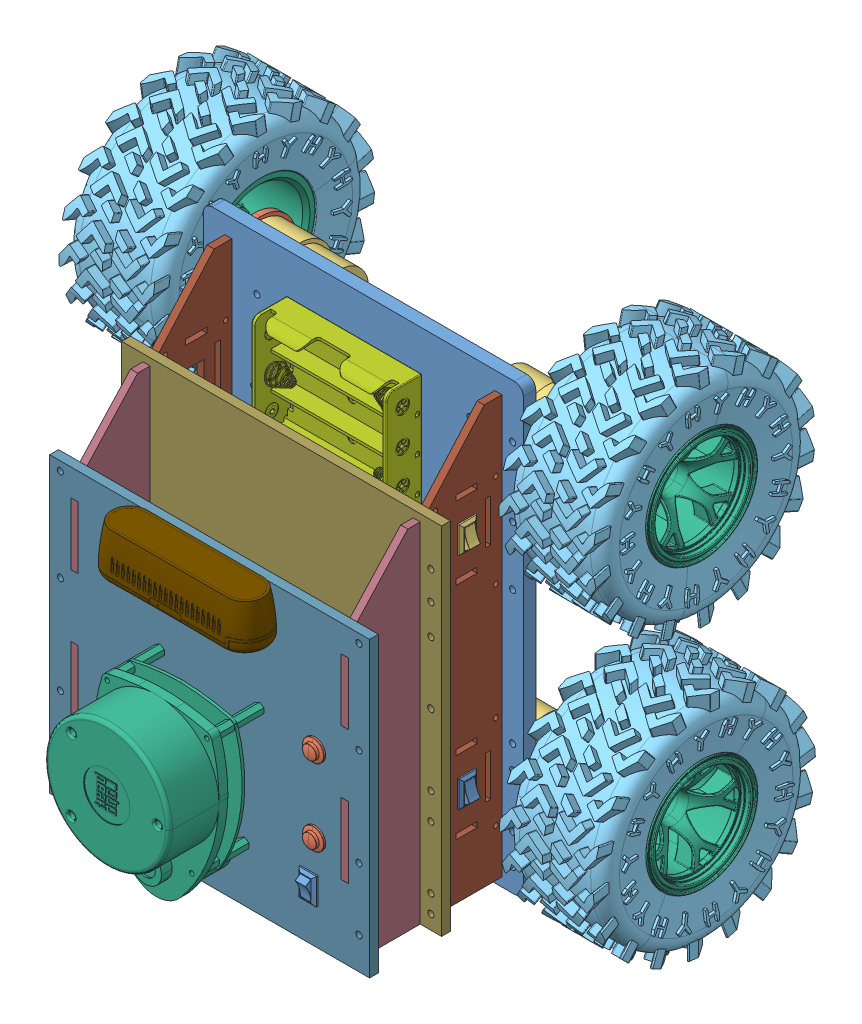
SolidWorks assembly Assem1, configuration Default. Lengths in mm.
Overall size (305.52 327.35 274.26).
98 component instances, 25 part files, 180 mates.
Components (placement in the parent):
- Tam_lot_motorLon-2: Tam_lot_motorLon [Default] at (-191.7952 1241.0975 -466.1522) size (180 250 7)
- thanh_dem_motor-12: thanh_dem_motor [Default] at (-373.0944 1216.0395 -541.7338) x (0.99999 -0.004493 0) z (0 0 1) size (43.51 40.52 47)
- thanh_dem_motor-13: thanh_dem_motor [Default] at (-373.0944 1056.0395 -541.7338) x (0.99999 -0.004493 0) z (0 0 1) size (43.51 40.52 47)
- thanh_dem_motor-14: thanh_dem_motor [Default] at (-10.496 1266.1855 -541.7338) x (-0.99999 0.004493 0) z (0 0 1) size (43.51 40.52 47)
- thanh_dem_motor-15: thanh_dem_motor [Default] at (-10.496 1426.1855 -541.7338) x (-0.99999 0.004493 0) z (0 0 1) size (43.51 40.52 47)
- Motor-12: Motor [Default] at (-348.7657 1055.9509 -541.5442) x (0.999999 -0.001679 0.000003) z (0 0.001679 0.999999) size (71.5 36.8 36.76)
- Motor-13: Motor [Default] at (-348.7657 1215.9559 -541.5442) x (0.999999 -0.001679 0.000003) z (0 0.001679 0.999999) size (71.5 36.8 36.76)
- Motor-14: Motor [Default] at (-34.8248 1266.2742 -541.5442) x (-0.999999 0.001679 0.000003) z (0 -0.001679 0.999999) size (71.5 36.8 36.76)
- Motor-15: Motor [Default] at (-34.8248 1426.2692 -541.5442) x (-0.999999 0.001679 0.000003) z (0 -0.001679 0.999999) size (71.5 36.8 36.76)
- Truc_noi_motor-12: Truc_noi_motor [Default] at (-342.5157 1166.658 -613.4496) x (0.999999 -0.000531 -0.001593) z (0 -0.948611 0.316446) size (18.27 12.66 13.76)
- Plastic Wheel 130mm-8: Plastic Wheel 130mm [Default] at (-67.9752 1161.396 -500.7246) x (1 0 0) z (0 -0.766044 0.642788) size (57.88 126.13 125.05)
  - Plastic Wheel 130mm.STEP-1: Plastic Wheel 130mm.STEP [Default] at origin size (57.88 126.13 125.05)
    - Tyre.STEP-1: Tyre.STEP [Default] at origin size (57.88 126.13 125.05)
    - Plastic Rim.STEP-1: Plastic Rim.STEP [Default] at (-24.3 0 0) x (0 -0.536317 -0.844017) z (0 -0.844017 0.536317) size (62 50 62)
- Plastic Wheel 130mm-10: Plastic Wheel 130mm [Default] at (-315.6152 1321.3029 -500.5854) x (-1 0 0) z (0 0.301603 -0.953434) size (57.88 126.13 125.05)
  - Plastic Wheel 130mm.STEP-1: Plastic Wheel 130mm.STEP [Default] at origin size (57.88 126.13 125.05)
    - Tyre.STEP-1: Tyre.STEP [Default] at origin size (57.88 126.13 125.05)
    - Plastic Rim.STEP-1: Plastic Rim.STEP [Default] at (-24.3 0 0) x (0 -0.536317 -0.844017) z (0 -0.844017 0.536317) size (62 50 62)
- Truc_noi_motor-14: Truc_noi_motor [Default] at (-41.0748 1219.1271 -452.682) x (-0.999999 -0.001675 0.000117) z (0 -0.069722 -0.997566) size (18.27 12.66 13.76)
- Plastic Wheel 130mm-11: Plastic Wheel 130mm [Default] at (-67.9752 1321.3326 -500.6086) x (1 0 0) z (0 -0.970088 0.242754) size (57.88 126.13 125.05)
  - Plastic Wheel 130mm.STEP-1: Plastic Wheel 130mm.STEP [Default] at origin size (57.88 126.13 125.05)
    - Tyre.STEP-1: Tyre.STEP [Default] at origin size (57.88 126.13 125.05)
    - Plastic Rim.STEP-1: Plastic Rim.STEP [Default] at (-24.3 0 0) x (0 -0.536317 -0.844017) z (0 -0.844017 0.536317) size (62 50 62)
- Truc_noi_motor-15: Truc_noi_motor [Default] at (-342.5157 1375.3924 -599.6649) x (0.999999 0.000219 -0.001665) z (0 -0.991439 -0.130574) size (18.27 12.66 13.76)
- Truc_noi_motor-16: Truc_noi_motor [Default] at (-41.0748 1098.7541 -406.8554) x (-0.999999 -0.001373 0.000967) z (0 -0.575859 -0.817549) size (18.27 12.66 13.76)
- Plastic Wheel 130mm-12: Plastic Wheel 130mm [Default] at (-315.6152 1161.399 -500.7183) x (-1 0 0) z (0 -0.235277 -0.971928) size (57.88 126.13 125.05)
  - Plastic Wheel 130mm.STEP-1: Plastic Wheel 130mm.STEP [Default] at origin size (57.88 126.13 125.05)
    - Tyre.STEP-1: Tyre.STEP [Default] at origin size (57.88 126.13 125.05)
    - Plastic Rim.STEP-1: Plastic Rim.STEP [Default] at (-24.3 0 0) x (0 -0.536317 -0.844017) z (0 -0.844017 0.536317) size (62 50 62)
- BTS_driver-2: BTS_driver [Default] at (-179.8452 1106.1475 -471.1522) x (0 1 0) z (0 0 -1) size (40.89 51.56 13.5)
- BTS_driver-3: BTS_driver [Default] at (-203.7452 1438.8875 -471.1522) x (0 -1 0) z (0 0 -1) size (40.89 51.56 13.5)
- BTS_driver-4: BTS_driver [Default] at (-203.7452 1376.0475 -471.1522) x (0 -1 0) z (0 0 -1) size (40.89 51.56 13.5)
- BTS_driver-5: BTS_driver [Default] at (-179.8452 1043.3075 -471.1522) x (0 1 0) z (0 0 -1) size (40.89 51.56 13.5)
- hexagone M3-1: hexagone M3 [Default] at (-145.1852 1312.4614 -471.1522) x (0 -1 0) z (1 0 0) size (5.78 5.38 5.01)
  - Assem_done(2)^hexagone M3-1: Assem_done(2)^hexagone M3 [Default] at origin size (5.78 5.38 5.01) (virtual)
    - hexagonal_spacer_FF_M3_H05_HEX5_pass_through.step^Assem_done(2)_hexagone M3-3: hexagonal_spacer_FF_M3_H05_HEX5_pass_through.step^Assem_done(2)_hexagone M3 [Default] at (22.1639 -5 15.1) x (1 0 0) z (0 1 0) size (5.78 5.01 5.38) (virtual)
- Copy of hexagonal_spacer_FF_M3_H05_HEX5_pass_through.step^Assem1-1: Copy of hexagonal_spacer_FF_M3_H05_HEX5_pass_through.step^Assem1 [Default] at (-175.8052 1254.7375 -466.1522) x (0 -1 0) z (0 0 -1) size (5.78 5.01 5.38) (virtual)
- Copy of hexagonal_spacer_FF_M3_H05_HEX5_pass_through.step^Assem1-2: Copy of hexagonal_spacer_FF_M3_H05_HEX5_pass_through.step^Assem1 [Default] at (-130.0852 1254.7375 -466.1522) x (0 -1 0) z (0 0 -1) size (5.78 5.01 5.38) (virtual)
- Copy of hexagonal_spacer_FF_M3_H05_HEX5_pass_through.step^Assem1-3: Copy of hexagonal_spacer_FF_M3_H05_HEX5_pass_through.step^Assem1 [Default] at (-175.8052 1290.2975 -466.1522) x (0 -1 0) z (0 0 -1) size (5.78 5.01 5.38) (virtual)
- Copy of hexagonal_spacer_FF_M3_H05_HEX5_pass_through.step^Assem1-4: Copy of hexagonal_spacer_FF_M3_H05_HEX5_pass_through.step^Assem1 [Default] at (-175.8052 1191.8975 -466.1522) x (0 -1 0) z (0 0 -1) size (5.78 5.01 5.38) (virtual)
- Copy of hexagonal_spacer_FF_M3_H05_HEX5_pass_through.step^Assem1-5: Copy of hexagonal_spacer_FF_M3_H05_HEX5_pass_through.step^Assem1 [Default] at (-175.8052 1227.4575 -466.1522) x (0 -1 0) z (0 0 -1) size (5.78 5.01 5.38) (virtual)
- Copy of hexagonal_spacer_FF_M3_H05_HEX5_pass_through.step^Assem1-6: Copy of hexagonal_spacer_FF_M3_H05_HEX5_pass_through.step^Assem1 [Default] at (-130.0852 1227.4575 -466.1522) x (0 -1 0) z (0 0 -1) size (5.78 5.01 5.38) (virtual)
- Copy of hexagonal_spacer_FF_M3_H05_HEX5_pass_through.step^Assem1-7: Copy of hexagonal_spacer_FF_M3_H05_HEX5_pass_through.step^Assem1 [Default] at (-130.0852 1191.8975 -466.1522) x (0 -1 0) z (0 0 -1) size (5.78 5.01 5.38) (virtual)
- Copy of hexagonal_spacer_FF_M3_H05_HEX5_pass_through.step^Assem1-9: Copy of hexagonal_spacer_FF_M3_H05_HEX5_pass_through.step^Assem1 [Default] at (-207.7852 1191.8975 -466.1522) x (0 -1 0) z (0 0 -1) size (5.78 5.01 5.38) (virtual)
- Copy of hexagonal_spacer_FF_M3_H05_HEX5_pass_through.step^Assem1-10: Copy of hexagonal_spacer_FF_M3_H05_HEX5_pass_through.step^Assem1 [Default] at (-253.5052 1254.7375 -466.1522) x (0 -1 0) z (0 0 -1) size (5.78 5.01 5.38) (virtual)
- Copy of hexagonal_spacer_FF_M3_H05_HEX5_pass_through.step^Assem1-11: Copy of hexagonal_spacer_FF_M3_H05_HEX5_pass_through.step^Assem1 [Default] at (-207.7852 1254.7375 -466.1522) x (0 -1 0) z (0 0 -1) size (5.78 5.01 5.38) (virtual)
- Copy of hexagonal_spacer_FF_M3_H05_HEX5_pass_through.step^Assem1-12: Copy of hexagonal_spacer_FF_M3_H05_HEX5_pass_through.step^Assem1 [Default] at (-207.7852 1290.2975 -466.1522) x (0 -1 0) z (0 0 -1) size (5.78 5.01 5.38) (virtual)
- Copy of hexagonal_spacer_FF_M3_H05_HEX5_pass_through.step^Assem1-13: Copy of hexagonal_spacer_FF_M3_H05_HEX5_pass_through.step^Assem1 [Default] at (-253.5052 1290.2975 -466.1522) x (0 -1 0) z (0 0 -1) size (5.78 5.01 5.38) (virtual)
- Copy of hexagonal_spacer_FF_M3_H05_HEX5_pass_through.step^Assem1-14: Copy of hexagonal_spacer_FF_M3_H05_HEX5_pass_through.step^Assem1 [Default] at (-207.7852 1227.4575 -466.1522) x (0 -1 0) z (0 0 -1) size (5.78 5.01 5.38) (virtual)
- Copy of hexagonal_spacer_FF_M3_H05_HEX5_pass_through.step^Assem1-15: Copy of hexagonal_spacer_FF_M3_H05_HEX5_pass_through.step^Assem1 [Default] at (-253.5052 1191.8975 -466.1522) x (0 -1 0) z (0 0 -1) size (5.78 5.01 5.38) (virtual)
- Copy of hexagonal_spacer_FF_M3_H05_HEX5_pass_through.step^Assem1-16: Copy of hexagonal_spacer_FF_M3_H05_HEX5_pass_through.step^Assem1 [Default] at (-253.5052 1227.4575 -466.1522) x (0 -1 0) z (0 0 -1) size (5.78 5.01 5.38) (virtual)
- Copy of hexagonal_spacer_FF_M3_H05_HEX5_pass_through.step^Assem1-17: Copy of hexagonal_spacer_FF_M3_H05_HEX5_pass_through.step^Assem1 [Default] at (-182.1594 1249.2225 -454.1522) x (0 -1 0) z (0 0 -1) size (5.78 5.01 5.38) (virtual)
- Copy of hexagonal_spacer_FF_M3_H05_HEX5_pass_through.step^Assem1-18: Copy of hexagonal_spacer_FF_M3_H05_HEX5_pass_through.step^Assem1 [Default] at (-202.0152 1232.9725 -454.1522) x (0 -1 0) z (0 0 -1) size (5.78 5.01 5.38) (virtual)
- Copy of hexagonal_spacer_FF_M3_H05_HEX5_pass_through.step^Assem1-21: Copy of hexagonal_spacer_FF_M3_H05_HEX5_pass_through.step^Assem1 [Default] at (-232.2152 1249.2225 -454.1522) x (0 -1 0) z (0 0 -1) size (5.78 5.01 5.38) (virtual)
- LM2596-3: LM2596 [Default] at (-217.1152 1255.1364 -459.1522) x (0 -1 0) z (1 0 0) size (21.25 15.15 43.2)
- LM2596-4: LM2596 [Default] at (-167.0594 1227.0586 -459.1522) x (0 1 0) z (-1 0 0) size (21.25 15.15 43.2)
- Copy of hexagonal_spacer_FF_M3_H05_HEX5_pass_through.step^Assem1-22: Copy of hexagonal_spacer_FF_M3_H05_HEX5_pass_through.step^Assem1 [Default] at (-151.9594 1232.9725 -454.1522) x (0 -1 0) z (0 0 -1) size (5.78 5.01 5.38) (virtual)
- mat_ben_co_sac-1: mat_ben_co_sac [Default] at (-269.7952 1238.5975 -459.1522) x (0 1 0) z (1 0 0) size (235 53 4)
- mat_ben_co_sac-2: mat_ben_co_sac [Default] at (-117.7952 1238.5975 -459.1522) x (0 1 0) z (1 0 0) size (235 53 4)
- tang2_2-2: tang2_2 [Default] at (-191.7952 1221.0975 -418.1522) x (0 1 0) z (0 0 1) size (200 180 5)
- mat_ben_tang_2-1: mat_ben_tang_2 [Default] at (-269.7952 1221.0975 -413.1522) x (0 1 0) z (1 0 0) size (196 45.5 4)
- mat_ben_tang_2-2: mat_ben_tang_2 [Default] at (-117.7952 1221.0975 -413.1522) x (0 1 0) z (1 0 0) size (196 45.5 4)
- tang_3-1: tang_3 [Default] at (-191.7952 1203.5975 -377.6522) x (-1 0 0) z (0 0 1) size (180 165 5)
- hexagone M3-2: hexagone M3 [Default] at (-182.3952 1137.4336 -409.1522) x (0 1 0) z (1 0 0) size (5.78 5.38 5.01)
  - Assem_done(2)^hexagone M3-1: Assem_done(2)^hexagone M3 [Default] at origin size (5.78 5.38 5.01) (virtual)
    - hexagonal_spacer_FF_M3_H05_HEX5_pass_through.step^Assem_done(2)_hexagone M3-3: hexagonal_spacer_FF_M3_H05_HEX5_pass_through.step^Assem_done(2)_hexagone M3 [Default] at (22.1639 -5 15.1) x (1 0 0) z (0 1 0) size (5.78 5.01 5.38) (virtual)
- Copy (2) of hexagonal_spacer_FF_M3_H05_HEX5_pass_through.step^Assem1-2: Copy (2) of hexagonal_spacer_FF_M3_H05_HEX5_pass_through.step^Assem1 [Default] at (-216.2952 1217.5975 -413.1522) x (0 1 0) z (0 0 1) size (5.78 5.01 5.38) (virtual)
- Copy (3) of hexagonal_spacer_FF_M3_H05_HEX5_pass_through.step^Assem1-3: Copy (3) of hexagonal_spacer_FF_M3_H05_HEX5_pass_through.step^Assem1 [Default] at (-216.2952 1159.5975 -413.9603) x (0 1 0) z (0 0 1) size (5.78 5.01 5.38) (virtual)
- Copy (4) of hexagonal_spacer_FF_M3_H05_HEX5_pass_through.step^Assem1-4: Copy (4) of hexagonal_spacer_FF_M3_H05_HEX5_pass_through.step^Assem1 [Default] at (-167.2952 1217.5975 -413.1522) x (0 1 0) z (0 0 1) size (5.78 5.01 5.38) (virtual)
- IntelRealsense_D435_Multibody-1: IntelRealsense_D435_Multibody [Default] at (-191.7952 1289.0475 -360.1522) x (-1 0 0) z (0 1 0) size (90.13 25.18 25.29)
- swith_on_off-1: swith_on_off [Default] at (-172.7952 1133.188 -448.951) x (0 1 0) z (1 0 0) size (15 10 19.96)
  - Assem_done(2)^swith_on_off-1: Assem_done(2)^swith_on_off [Default] at origin size (15 10 19.96) (virtual)
    - Switch on off^Assem_done(2)_swith_on_off-1: Switch on off^Assem_done(2)_swith_on_off [Default] at (40.9627 9.8337 51) x (0 1 0) z (1 0 0) size (10 19.96 15) (virtual)
- swith_hold-2: swith_hold [Default] at (-104.7178 1093.4107 -443.6522) x (0 1 0) z (1 0 0) size (12.02 24.8 12.02)
  - Assem_done(2)^swith_hold-1: Assem_done(2)^swith_hold [Default] at origin size (12.02 24.8 12.02) (virtual)
    - Push_main_Défaut^Assem_done(2)_swith_hold-1: Push_main_Défaut^Assem_done(2)_swith_hold [Default] at (80.7059 56 -27.817) size (12.02 24.8 12.02) (virtual)
- swith_hold-3: swith_hold [Default] at (-104.7178 1136.5135 -443.6522) x (0 1 0) z (1 0 0) size (12.02 24.8 12.02)
  - Assem_done(2)^swith_hold-1: Assem_done(2)^swith_hold [Default] at origin size (12.02 24.8 12.02) (virtual)
    - Push_main_Défaut^Assem_done(2)_swith_hold-1: Push_main_Défaut^Assem_done(2)_swith_hold [Default] at (80.7059 56 -27.817) size (12.02 24.8 12.02) (virtual)
- Copy of Switch on off^Assem1-1: Copy of Switch on off^Assem1 [Default] at (-121.7952 1298.0058 -439.1172) x (0 0 1) z (0 1 0) size (10 19.96 15) (virtual)
- raspberry pi 4-2: raspberry pi 4 [Default] at (-177.8669 1229.5402 -448.1622) x (0 -1 0) z (-1 0 0) size (89 19.92 58.4)
  - Assem_done(2)^raspberry pi 4-1: Assem_done(2)^raspberry pi 4 [Default] at origin size (89 19.92 58.4) (virtual)
    - Raspberry Pi 4 Model B^Assem_done(2)_raspberry pi 4-1: Raspberry Pi 4 Model B^Assem_done(2)_raspberry pi 4 [Default] at (50.9427 40.8 13.9283) size (89 19.92 58.4) (virtual)
- LM2596-5: LM2596 [Default] at (-155.8342 1158.5975 -413.1522) x (1 0 0) z (0 1 0) size (21.25 15.15 43.2)
- Copy (5) of hexagonal_spacer_FF_M3_H05_HEX5_pass_through.step^Assem1-1: Copy (5) of hexagonal_spacer_FF_M3_H05_HEX5_pass_through.step^Assem1 [Default] at (-133.6702 1173.6975 -413.1522) x (-1 0 0) z (0 0 1) size (5.78 5.01 5.38) (virtual)
- Copy (5) of hexagonal_spacer_FF_M3_H05_HEX5_pass_through.step^Assem1-2: Copy (5) of hexagonal_spacer_FF_M3_H05_HEX5_pass_through.step^Assem1 [Default] at (-149.9202 1143.4975 -413.1522) x (-1 0 0) z (0 0 1) size (5.78 5.01 5.38) (virtual)
- lidarA1-2: lidarA1 [Default] at (-193.9966 1206.7256 -443.6522) x (0 1 0) z (1 0 0) size (98.94 57.7 70.63)
  - Assem_done(2)^lidarA1-1: Assem_done(2)^lidarA1 [Default] at origin size (98.94 57.7 70.63) (virtual)
    - rplidar_main_По умолчанию^Assem_done(2)_lidarA1-1: rplidar_main_По умолчанию^Assem_done(2)_lidarA1 [Default] at (-27.1712 95.6 1.9102) x (-0.99998 0 -0.006299) z (0.006299 0 -0.99998) size (98.5 57.7 70.02) (virtual)
- swith_on_off-2: swith_on_off [Default] at (-145.664 1189.9255 -431.6522) x (0 -1 0) z (0 0 1) size (15 10 19.96)
  - Assem_done(2)^swith_on_off-1: Assem_done(2)^swith_on_off [Default] at origin size (15 10 19.96) (virtual)
    - Switch on off^Assem_done(2)_swith_on_off-1: Switch on off^Assem_done(2)_swith_on_off [Default] at (40.9627 9.8337 51) x (0 1 0) z (1 0 0) size (10 19.96 15) (virtual)
- Copy of hexagonal_spacer_FF_M3_H05_HEX5_pass_through.step^Assem1-33: Copy of hexagonal_spacer_FF_M3_H05_HEX5_pass_through.step^Assem1 [Default] at (-191.7952 1202.4375 -454.1522) x (0 -1 0) z (0 0 -1) size (5.78 5.01 5.38) (virtual)
- Copy of hexagonal_spacer_FF_M3_H05_HEX5_pass_through.step^Assem1-34: Copy of hexagonal_spacer_FF_M3_H05_HEX5_pass_through.step^Assem1 [Default] at (-191.7952 1279.7575 -454.1522) x (0 -1 0) z (0 0 -1) size (5.78 5.01 5.38) (virtual)
- Copy of hexagonal_spacer_FF_M3_H05_HEX5_pass_through.step^Assem1-35: Copy of hexagonal_spacer_FF_M3_H05_HEX5_pass_through.step^Assem1 [Default] at (-191.7952 1338.2575 -454.1522) x (0 -1 0) z (0 0 -1) size (5.78 5.01 5.38) (virtual)
- Copy of hexagonal_spacer_FF_M3_H05_HEX5_pass_through.step^Assem1-36: Copy of hexagonal_spacer_FF_M3_H05_HEX5_pass_through.step^Assem1 [Default] at (-191.7952 1143.9375 -454.1522) x (0 -1 0) z (0 0 -1) size (5.78 5.01 5.38) (virtual)
- 18650 Battery Holder 4x-2: 18650 Battery Holder 4x [Default] at (-191.7952 1279.7575 -444.1522) x (0 1 0) z (1 0 0) size (99.89 20 92.22)
- 18650 Battery Holder 4x-3: 18650 Battery Holder 4x [Default] at (-191.7952 1143.9375 -444.1522) x (0 1 0) z (1 0 0) size (99.89 20 92.22)
Mates (geometry in assembly coordinates):
- Coincident62: coincident anti-aligned: plane of Tam_lot_motorLon-2 through (-191.7952 1241.0975 -466.1522) normal (0 0 -1); plane of thanh_dem_motor-12 through (-236.0722 1348.0787 -466.1522) normal (0 0 1)
- Parallel22: parallel aligned: plane of Tam_lot_motorLon-2 through (-281.7952 1366.0975 -459.1522) normal (-1 0 0); plane of thanh_dem_motor-12 through (-286.8552 1300.9375 -513.1522) normal (-1 0 0)
- Coincident64: coincident anti-aligned: plane of Tam_lot_motorLon-2 through (-191.7952 1241.0975 -466.1522) normal (0 0 -1); plane of thanh_dem_motor-13 through (-236.0722 1188.0787 -466.1522) normal (0 0 1)
- Parallel23: parallel aligned: plane of Tam_lot_motorLon-2 through (-281.7952 1366.0975 -459.1522) normal (-1 0 0); plane of thanh_dem_motor-13 through (-286.8552 1140.9375 -513.1522) normal (-1 0 0)
- Coincident66: coincident anti-aligned: plane of Tam_lot_motorLon-2 through (-191.7952 1241.0975 -466.1522) normal (0 0 -1); plane of thanh_dem_motor-14 through (-147.5183 1134.1463 -466.1522) normal (0 0 1)
- Parallel24: parallel aligned: plane of Tam_lot_motorLon-2 through (-101.7952 1366.0975 -459.1522) normal (1 0 0); plane of thanh_dem_motor-14 through (-96.7352 1181.2875 -513.1522) normal (1 0 0)
- Coincident68: coincident anti-aligned: plane of Tam_lot_motorLon-2 through (-191.7952 1241.0975 -466.1522) normal (0 0 -1); plane of thanh_dem_motor-15 through (-147.5183 1294.1463 -466.1522) normal (0 0 1)
- Parallel25: parallel aligned: plane of Tam_lot_motorLon-2 through (-101.7952 1366.0975 -459.1522) normal (1 0 0); plane of thanh_dem_motor-15 through (-96.7352 1341.2875 -513.1522) normal (1 0 0)
- Coincident70: coincident anti-aligned: circle of thanh_dem_motor-14; circle of Motor-12
- Concentric56: concentric aligned: cylinder of thanh_dem_motor-14 through (-198.7352 1168.9125 -506.4295) axis (1 0 0) radius 1.55; cylinder of Motor-12 through (-103.1852 1168.9125 -506.4295) axis (1 0 0) radius 1.255
- Parallel27: parallel aligned: plane of thanh_dem_motor-14 through (-147.5183 1079.2875 -469.6022) normal (0 0 -1); plane of Motor-12 through (-91.5252 1163.1665 -503.3051) normal (0 0 -1)
- Coincident72: coincident anti-aligned: plane of thanh_dem_motor-13 through (-283.4052 1242.9375 -466.1522) normal (1 0 0); plane of Motor-14 through (-283.4052 1161.115 -492.9151) normal (-1 0 0)
- Concentric59: concentric aligned: cylinder of thanh_dem_motor-13 through (-184.8552 1153.3125 -506.4295) axis (-1 0 0) radius 1.55; cylinder of Motor-14 through (-280.4052 1153.3125 -506.4295) axis (-1 0 0) radius 1.255
- Parallel28: parallel aligned: plane of thanh_dem_motor-13 through (-236.0722 1242.9375 -469.6022) normal (0 0 -1); plane of Motor-14 through (-292.0652 1159.0585 -503.3051) normal (0 0 -1)
- Coincident74: coincident aligned: plane of thanh_dem_motor-12 through (-283.4052 1402.9375 -466.1522) normal (1 0 0); circle of Motor-15
- Concentric60: concentric aligned: cylinder of thanh_dem_motor-12 through (-184.8552 1328.9125 -506.4295) axis (-1 0 0) radius 1.55; cylinder of Motor-15 through (-280.4052 1328.9125 -506.4295) axis (-1 0 0) radius 1.255
- Parallel29: parallel aligned: plane of thanh_dem_motor-12 through (-236.0722 1402.9375 -469.6022) normal (0 0 -1); plane of Motor-15 through (-292.0652 1319.0535 -503.3051) normal (0 0 -1)
- Coincident76: coincident anti-aligned: plane of thanh_dem_motor-15 through (-100.1852 1239.2875 -466.1522) normal (-1 0 0); plane of Motor-13 through (-100.1852 1321.115 -492.9151) normal (1 0 0)
- Concentric61: concentric aligned: cylinder of thanh_dem_motor-15 through (-198.7352 1313.3125 -506.4295) axis (1 0 0) radius 1.55; cylinder of Motor-13 through (-103.1852 1313.3125 -506.4295) axis (1 0 0) radius 1.255
- Parallel30: parallel aligned: plane of thanh_dem_motor-15 through (-147.5183 1239.2875 -469.6022) normal (0 0 -1); plane of Motor-13 through (-91.5252 1323.1715 -503.3051) normal (0 0 -1)
- Coincident79: coincident anti-aligned: plane of Truc_noi_motor-12 through (-73.2752 1159.0538 -494.3201) normal (1 0 0); plane of Plastic Wheel 130mm-8/Plastic Wheel 130mm.STEP-1/Plastic Rim.STEP-1 through (-73.2752 1161.396 -500.7246) normal (-1 0 0)
- Parallel31: parallel anti-aligned: plane of Truc_noi_motor-12 through (-91.5252 1159.0754 -494.2225) normal (0 0.215302 0.976548); plane of Plastic Wheel 130mm-8/Plastic Wheel 130mm.STEP-1/Plastic Rim.STEP-1 through (-73.2752 1159.2527 -493.9544) normal (0 -0.215302 -0.976548)
- Coincident81: coincident anti-aligned: plane of Truc_noi_motor-12 through (-91.5252 1154.3833 -499.2809) normal (0 -0.738064 0.674731); plane of Plastic Wheel 130mm-8/Plastic Wheel 130mm.STEP-1/Plastic Rim.STEP-1 through (-73.2752 1154.4612 -499.1957) normal (0 0.738064 -0.674731)
- Coincident82: coincident anti-aligned: plane of Truc_noi_motor-12 through (-91.5252 1163.1447 -507.4078) normal (0 -0.215302 -0.976548); plane of Plastic Wheel 130mm-8/Plastic Wheel 130mm.STEP-1/Plastic Rim.STEP-1 through (-73.2752 1163.5394 -507.4948) normal (0 0.215302 0.976548)
- Coincident86: coincident anti-aligned: plane of Plastic Wheel 130mm-10/Plastic Wheel 130mm.STEP-1/Plastic Rim.STEP-1 through (-310.3152 1315.8639 -496.0195) normal (0 0.984769 -0.173869); plane of Truc_noi_motor-14 through (-292.0652 1315.7937 -496.4174) normal (0 -0.984769 0.173869)
- Coincident87: coincident anti-aligned: plane of Plastic Wheel 130mm-10/Plastic Wheel 130mm.STEP-1/Plastic Rim.STEP-1 through (-310.3152 1321.3029 -500.5854) normal (1 0 0); plane of Truc_noi_motor-14 through (-310.3152 1326.3279 -505.1955) normal (-1 0 0)
- Coincident88: coincident anti-aligned: plane of Plastic Wheel 130mm-10/Plastic Wheel 130mm.STEP-1/Plastic Rim.STEP-1 through (-310.3152 1320.0682 -507.5786) normal (0 -0.341809 0.939769); plane of Truc_noi_motor-14 through (-292.0652 1319.9597 -507.6181) normal (0 0.341809 -0.939769)
- Parallel33: parallel anti-aligned: plane of Plastic Wheel 130mm-10/Plastic Wheel 130mm.STEP-1/Plastic Rim.STEP-1 through (-310.3152 1326.7419 -505.1513) normal (0 -0.984769 0.173869); plane of Truc_noi_motor-14 through (-292.0652 1326.4264 -505.2128) normal (0 0.984769 -0.173869)
- Coincident89: coincident anti-aligned: plane of Plastic Wheel 130mm-11/Plastic Wheel 130mm.STEP-1/Plastic Rim.STEP-1 through (-73.2752 1326.2224 -505.7582) normal (0 -0.233744 0.972298); plane of Truc_noi_motor-15 through (-91.5252 1325.8295 -505.8527) normal (0 0.233744 -0.972298)
- Coincident90: coincident anti-aligned: plane of Plastic Wheel 130mm-11/Plastic Wheel 130mm.STEP-1/Plastic Rim.STEP-1 through (-73.2752 1321.3326 -500.6086) normal (-1 0 0); plane of Truc_noi_motor-15 through (-73.2752 1316.4239 -495.8748) normal (1 0 0)
- Coincident91: coincident anti-aligned: plane of Plastic Wheel 130mm-11/Plastic Wheel 130mm.STEP-1/Plastic Rim.STEP-1 through (-73.2752 1314.4279 -502.2685) normal (0 0.958907 -0.283721); plane of Truc_noi_motor-15 through (-91.5252 1314.3951 -502.3792) normal (0 -0.958907 0.283721)
- Parallel34: parallel anti-aligned: plane of Plastic Wheel 130mm-11/Plastic Wheel 130mm.STEP-1/Plastic Rim.STEP-1 through (-73.2752 1316.4427 -495.4589) normal (0 0.233744 -0.972298); plane of Truc_noi_motor-15 through (-91.5252 1316.4006 -495.7776) normal (0 -0.233744 0.972298)
- Concentric62: concentric aligned: cylinder of Motor-13 through (-79.5252 1321.115 -500.8151) axis (-1 0 0) radius 3; cylinder of Truc_noi_motor-15 through (-68.6083 1321.115 -500.8151) axis (-1 0 0) radius 1.5
- Coincident92: coincident anti-aligned: plane of Motor-13 through (-91.5252 1321.115 -492.9151) normal (1 0 0); plane of Truc_noi_motor-15 through (-91.5252 1316.4239 -495.8748) normal (-1 0 0)
- Concentric63: concentric aligned: cylinder of Motor-12 through (-79.5252 1161.11 -500.8151) axis (-1 0 0) radius 3; cylinder of Truc_noi_motor-12 through (-68.6083 1161.11 -500.8151) axis (-1 0 0) radius 1.5
- Coincident93: coincident anti-aligned: plane of Motor-12 through (-91.5252 1161.11 -492.9151) normal (1 0 0); circle of Truc_noi_motor-12
- Coincident97: coincident anti-aligned: plane of Truc_noi_motor-16 through (-292.0652 1156.6104 -506.0412) normal (0 -0.193801 -0.981041); plane of Plastic Wheel 130mm-12/Plastic Wheel 130mm.STEP-1/Plastic Rim.STEP-1 through (-310.3152 1156.7237 -506.0636) normal (0 0.193801 0.981041)
- Coincident98: coincident anti-aligned: plane of Truc_noi_motor-16 through (-310.3152 1163.3134 -507.2634) normal (-1 0 0); plane of Plastic Wheel 130mm-12/Plastic Wheel 130mm.STEP-1/Plastic Rim.STEP-1 through (-310.3152 1161.399 -500.7183) normal (1 0 0)
- Coincident99: coincident anti-aligned: plane of Truc_noi_motor-16 through (-292.0652 1158.8414 -494.301) normal (0 -0.752706 0.658357); plane of Plastic Wheel 130mm-12/Plastic Wheel 130mm.STEP-1/Plastic Rim.STEP-1 through (-310.3152 1159.1075 -493.9968) normal (0 0.752706 -0.658357)
- Parallel35: parallel anti-aligned: plane of Truc_noi_motor-16 through (-292.0652 1163.3887 -507.3293) normal (0 0.752706 -0.658357); plane of Plastic Wheel 130mm-12/Plastic Wheel 130mm.STEP-1/Plastic Rim.STEP-1 through (-310.3152 1163.6905 -507.4399) normal (0 -0.752706 0.658357)
- Concentric64: concentric aligned: cylinder of Motor-15 through (-304.0652 1321.11 -500.8151) axis (1 0 0) radius 3; cylinder of Truc_noi_motor-14 through (-314.9821 1321.11 -500.8151) axis (1 0 0) radius 1.5
- Coincident101: coincident anti-aligned: plane of Motor-15 through (-292.0652 1321.11 -492.9151) normal (-1 0 0); plane of Truc_noi_motor-14 through (-292.0652 1326.3279 -505.1955) normal (1 0 0)
- Concentric65: concentric aligned: cylinder of Motor-14 through (-304.0652 1161.115 -500.8151) axis (1 0 0) radius 3; cylinder of Truc_noi_motor-16 through (-314.9821 1161.115 -500.8151) axis (1 0 0) radius 1.5
- Coincident102: coincident anti-aligned: plane of Motor-14 through (-292.0652 1161.115 -492.9151) normal (-1 0 0); plane of Truc_noi_motor-16 through (-292.0652 1163.3134 -507.2634) normal (1 0 0)
- Coincident103: coincident anti-aligned: plane of Tam_lot_motorLon-2 through (-191.7952 1241.0975 -459.1522) normal (0 0 1); plane of khay_pin-4/Assem_done(2)^khay_pin-1/18650 Cell Holder^Assem_done(2)_khay_pin-1 through (-191.7952 1302.6325 -459.1522) normal (0 0 -1)
- Concentric68: concentric anti-aligned: cylinder of Tam_lot_motorLon-2 through (-251.7352 1336.0575 -454.2591) axis (0 0 -1) radius 1.73; cylinder of thanh_dem_motor-12 through (-251.7352 1336.0575 -571.6022) axis (0 0 1) radius 1.73
- Concentric69: concentric anti-aligned: cylinder of Tam_lot_motorLon-2 through (-251.7352 1176.0575 -454.2591) axis (0 0 -1) radius 1.73; cylinder of thanh_dem_motor-13 through (-251.7352 1176.0575 -571.6022) axis (0 0 1) radius 1.73
- Concentric70: concentric anti-aligned: cylinder of Tam_lot_motorLon-2 through (-131.8552 1336.0575 -454.2591) axis (0 0 -1) radius 1.73; cylinder of thanh_dem_motor-15 through (-131.8552 1336.0575 -571.6022) axis (0 0 1) radius 1.73
- Concentric71: concentric anti-aligned: cylinder of Tam_lot_motorLon-2 through (-131.8552 1176.0575 -454.2591) axis (0 0 -1) radius 1.73; cylinder of thanh_dem_motor-14 through (-131.8552 1176.0575 -571.6022) axis (0 0 1) radius 1.73
- Concentric72: concentric anti-aligned: cylinder of BTS_driver-3 through (-175.8052 1290.2975 -470.3622) axis (0 0 -1) radius 1.75; cylinder of Copy of hexagonal_spacer_FF_M3_H05_HEX5_pass_through.step^Assem1-3 through (-175.8052 1290.2975 -470.8751) axis (0 0 1) radius 1.5
- Coincident104: coincident anti-aligned: plane of BTS_driver-3 through (-152.8182 1272.3905 -471.1522) normal (0 0 1); plane of Copy of hexagonal_spacer_FF_M3_H05_HEX5_pass_through.step^Assem1-3 through (-175.8052 1290.2975 -471.1522) normal (0 0 -1)
- Concentric73: concentric anti-aligned: cylinder of BTS_driver-3 through (-175.8052 1254.7375 -470.3622) axis (0 0 -1) radius 1.75; cylinder of Copy of hexagonal_spacer_FF_M3_H05_HEX5_pass_through.step^Assem1-1 through (-175.8052 1254.7375 -470.8751) axis (0 0 1) radius 1.5
- Coincident105: coincident anti-aligned: plane of BTS_driver-3 through (-152.8182 1272.3905 -471.1522) normal (0 0 1); plane of Copy of hexagonal_spacer_FF_M3_H05_HEX5_pass_through.step^Assem1-1 through (-175.8052 1254.7375 -471.1522) normal (0 0 -1)
- Concentric74: concentric anti-aligned: cylinder of BTS_driver-3 through (-130.0852 1254.7375 -470.3622) axis (0 0 -1) radius 1.75; cylinder of Copy of hexagonal_spacer_FF_M3_H05_HEX5_pass_through.step^Assem1-2 through (-130.0852 1254.7375 -470.8751) axis (0 0 1) radius 1.5
- Coincident106: coincident anti-aligned: plane of BTS_driver-3 through (-152.8182 1272.3905 -471.1522) normal (0 0 1); plane of Copy of hexagonal_spacer_FF_M3_H05_HEX5_pass_through.step^Assem1-2 through (-130.0852 1254.7375 -471.1522) normal (0 0 -1)
- Concentric75: concentric anti-aligned: cylinder of BTS_driver-3 through (-130.0852 1290.2975 -470.3622) axis (0 0 -1) radius 1.75; cylinder of hexagone M3-1/Assem_done(2)^hexagone M3-1/hexagonal_spacer_FF_M3_H05_HEX5_pass_through.step^Assem_done(2)_hexagone M3-3 through (-130.0852 1290.2975 -470.8751) axis (0 0 1) radius 1.5
- Coincident107: coincident anti-aligned: plane of BTS_driver-3 through (-152.8182 1272.3905 -471.1522) normal (0 0 1); plane of hexagone M3-1/Assem_done(2)^hexagone M3-1/hexagonal_spacer_FF_M3_H05_HEX5_pass_through.step^Assem_done(2)_hexagone M3-3 through (-130.0852 1290.2975 -471.1522) normal (0 0 -1)
- Concentric76: concentric anti-aligned: cylinder of BTS_driver-4 through (-175.8052 1191.8975 -470.3622) axis (0 0 -1) radius 1.75; cylinder of Copy of hexagonal_spacer_FF_M3_H05_HEX5_pass_through.step^Assem1-4 through (-175.8052 1191.8975 -470.8751) axis (0 0 1) radius 1.5
